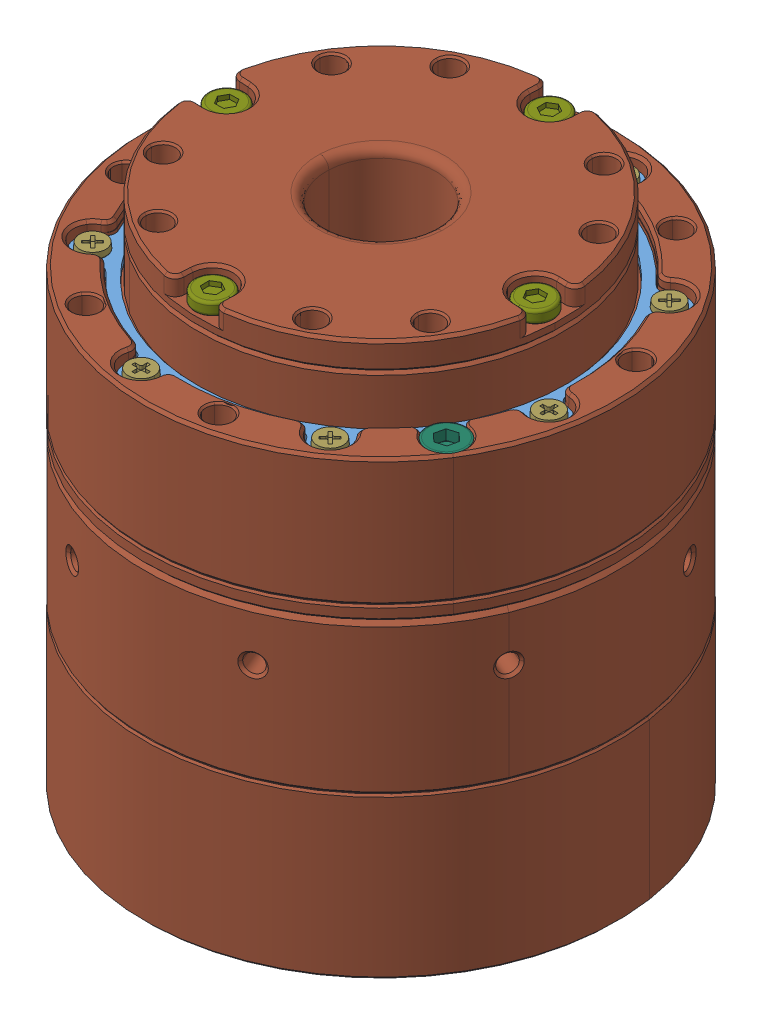
SolidWorks assembly CRA-RI40-52-PRO-XX 2023.5.4 - Drum, configuration 默认. Lengths in mm.
Overall size (67.95 60.31 67.96).
56 component instances, 34 part files, 0 mates.
Components (placement in the parent):
- CRA-RI40-52-PRO-XX 2023.5.4 - Drum.stp-1: CRA-RI40-52-PRO-XX 2023.5.4 - Drum.stp [默认] at origin size (67.95 60.31 67.96)
  - CRA-RI40-52-PRO-XX_1_ASM.stp-1: CRA-RI40-52-PRO-XX_1_ASM.stp [默认] at origin size (67.95 60.31 67.96)
    - XB11-52__10001_ASM.stp-1: XB11-52__10001_ASM.stp [默认] at (0 16.8 0) x (0.703875 0 -0.710324) z (-0.710324 0 -0.703875) size (66.32 0.8 66.32)
      - XB11-52-06__10001.stp-1: XB11-52-06__10001.stp [默认] at (0 15.8 0) x (0.791272 0 -0.611464) z (-0.611464 0 -0.791272) size (47.28 0.81 47.28)
    - TINYMBS20WITHCONNECTOR2_ASM.stp-1: TINYMBS20WITHCONNECTOR2_ASM.stp [默认] at (2.7275 -27.9719 -6.5848) x (0 -1 0) z (0.92388 0 0.382683) size (0.82 3.25 5.53)
      - FH34SRJ8S05SH_STEP_STEP_ASM.stp-1: FH34SRJ8S05SH_STEP_STEP_ASM.stp [默认] at (-6.4719 -22.2833 0) x (0 0 -1) z (1 0 0) size (5.53 3.25 0.82)
        - NONE-51348.stp-1: NONE-51348.stp [默认] at origin size (0.15 0.3 0.08)
        - NONE-53783.stp-1: NONE-53783.stp [默认] at origin size (0.15 0.3 0.08)
        - NONE-55744.stp-1: NONE-55744.stp [默认] at origin size (0.15 0.08 0.08)
        - NONE-57763.stp-1: NONE-57763.stp [默认] at origin size (0.15 0.08 0.08)
        - NONE-60582.stp-1: NONE-60582.stp [默认] at origin size (0.15 0.3 0.08)
        - NONE-60979.stp-1: NONE-60979.stp [默认] at origin size (0.15 0.3 0.08)
        - NONE-62950.stp-1: NONE-62950.stp [默认] at origin size (0.15 0.3 0.08)
        - NONE-64179.stp-1: NONE-64179.stp [默认] at origin size (0.15 0.3 0.08)
        - NONE-65774.stp-1: NONE-65774.stp [默认] at origin size (0.15 0.08 0.08)
        - NONE-66548.stp-1: NONE-66548.stp [默认] at origin size (0.15 0.35 0.23)
        - NONE-67775.stp-1: NONE-67775.stp [默认] at origin size (0.15 0.35 0.23)
        - NONE-133224.stp-1: NONE-133224.stp [默认] at origin size (0.15 0.08 0.08)
        - NONE-134873.stp-1: NONE-134873.stp [默认] at origin size (0.15 0.3 0.08)
        - NONE-136443.stp-1: NONE-136443.stp [默认] at origin size (0.15 0.08 0.08)
        - NONE-141250.stp-1: NONE-141250.stp [默认] at origin size (0.15 0.35 0.23)
        - NONE-145287.stp-1: NONE-145287.stp [默认] at origin size (0.15 0.08 0.08)
        - NONE-147294.stp-1: NONE-147294.stp [默认] at origin size (0.15 0.08 0.08)
        - NONE-214429.stp-1: NONE-214429.stp [默认] at origin size (0.15 0.9 0.82)
        - NONE-214822.stp-1: NONE-214822.stp [默认] at origin size (0.15 0.3 0.08)
        - NONE-215190.stp-1: NONE-215190.stp [默认] at origin size (0.15 0.08 0.08)
        - NONE-216041.stp-1: NONE-216041.stp [默认] at origin size (0.15 0.35 0.23)
        - NONE-217624.stp-1: NONE-217624.stp [默认] at origin size (0.15 0.35 0.23)
        - NONE-222885.stp-1: NONE-222885.stp [默认] at origin size (0.15 0.35 0.23)
        - NONE-224875.stp-1: NONE-224875.stp [默认] at origin size (0.15 0.35 0.23)
        - NONE-228113.stp-1: NONE-228113.stp [默认] at origin size (0.15 0.9 0.82)
        - NONE-228916.stp-1: NONE-228916.stp [默认] at origin size (0.15 0.35 0.23)
    - CROSS_RECESSED_COUNTERSUNK_HE_1.stp-1: CROSS_RECESSED_COUNTERSUNK_HE_1.stp [默认] at (-21.8123 -33.1 2.8703) x (0 1 0) z (0.6 0 0.8) size (4 3.5 3.5)
    - RI40-52-D12-02__1000.stp-1: RI40-52-D12-02__1000.stp [默认] at (0 -15 0) x (0.382683 0 -0.92388) z (0.92388 0 0.382683) size (52.01 56.6 52)
    - CROSS_RECESSED_CHEESE_HEAD_SC_1.stp-1: CROSS_RECESSED_CHEESE_HEAD_SC_1.stp [默认] at (3.9505 15.5 -22.4044) x (0 -1 0) z (1 0 0) size (5.7 2.98 2.98)
    - MC50-D25X12_5_000.stp-1: MC50-D25X12_5_000.stp [默认] at (0.0001 -26.6014 0.0001) x (0.382686 0 -0.923879) z (0 -1 0) size (48.11 50.01 13.43)
    - CROSS_RECESSED_CHEESE_HEAD_SC_1.stp-2: CROSS_RECESSED_CHEESE_HEAD_SC_1.stp [默认] at (-3.9505 15.5 22.4044) x (0 -1 0) z (-1 0 0) size (5.7 2.98 2.98)
    - CROSS_RECESSED_COUNTERSUNK_HE_1.stp-2: CROSS_RECESSED_COUNTERSUNK_HE_1.stp [默认] at (-3.0048 -33.1 22.5417) x (0 1 0) z (0.395734 0 0.918365) size (4 3.5 3.5)
    - CROSS_RECESSED_CHEESE_HEAD_SC_1.stp-3: CROSS_RECESSED_CHEESE_HEAD_SC_1.stp [默认] at (-18.6357 15.5 13.0489) x (0 -1 0) z (-0.707107 0 -0.707107) size (5.7 2.98 2.98)
    - CROSS_RECESSED_COUNTERSUNK_HE_1.stp-3: CROSS_RECESSED_COUNTERSUNK_HE_1.stp [默认] at (18.8645 -33.1 -12.4259) x (0 1 0) z (0.188455 0 0.982082) size (4 3.5 3.5)
    - _M2X3_M2X3_100.stp-1: _M2X3_M2X3_100.stp [默认] at (-21.8118 -29.6014 2.8705) x (0.8 0 -0.6) z (0.6 0 0.8) size (3.23 5.8 2.8)
    - _M2X3_M2X3_100.stp-2: _M2X3_M2X3_100.stp [默认] at (-13.393 -29.6014 -17.4539) x (0.918365 0 -0.395734) z (0.395734 0 0.918365) size (3.23 5.8 2.8)
    - CROSS_RECESSED_CHEESE_HEAD_SC_1.stp-4: CROSS_RECESSED_CHEESE_HEAD_SC_1.stp [默认] at (-22.4044 15.5 -3.9505) x (0 -1 0) z (0 0 -1) size (5.7 2.98 2.98)
    - CROSS_RECESSED_CHEESE_HEAD_SC_1.stp-5: CROSS_RECESSED_CHEESE_HEAD_SC_1.stp [默认] at (13.0489 15.5 18.6357) x (0 -1 0) z (-0.707107 0 0.707107) size (5.7 2.98 2.98)
    - HEXAGON_SOCKET_HEAD_CAP_SCREW_1.stp-1: HEXAGON_SOCKET_HEAD_CAP_SCREW_1.stp [默认] at (19.8197 15.9 12.6265) x (0 -1 0) z (-0.954517 0 0.298155) size (22.5 4.5 4.5)
    - M2-3_10001.stp-1: M2-3_10001.stp [默认] at (0.7742 21 -17.7331) x (0.020141 0 0.999797) z (-0.999797 0 0.020141) size (4 5.4 4)
    - HEXAGON_SOCKET_HEAD_CAP_SCREW_1.stp-2: HEXAGON_SOCKET_HEAD_CAP_SCREW_1.stp [默认] at (-19.8197 15.9 -12.6265) x (0 -1 0) z (0.954517 0 -0.298155) size (22.5 4.5 4.5)
    - CROSS_RECESSED_CHEESE_HEAD_SC_1.stp-6: CROSS_RECESSED_CHEESE_HEAD_SC_1.stp [默认] at (18.6357 15.5 -13.0489) x (0 -1 0) z (0.707107 0 0.707107) size (5.7 2.98 2.98)
    - M2-3_10001.stp-2: M2-3_10001.stp [默认] at (-17.7331 21 -0.7742) x (0.999797 0 -0.020141) z (0.020141 0 0.999797) size (4 5.4 4)
    - _M2X3_M2X3_100.stp-3: _M2X3_M2X3_100.stp [默认] at (-3.0038 -29.6014 22.5414) x (0.982082 0 -0.188455) z (0.188455 0 0.982082) size (3.23 5.8 2.8)
    - M2-3_10001.stp-3: M2-3_10001.stp [默认] at (-0.7742 21 17.7331) x (-0.020141 0 -0.999797) z (0.999797 0 -0.020141) size (4 5.4 4)
    - _M2X3_M2X3_100.stp-4: _M2X3_M2X3_100.stp [默认] at (18.8646 -29.6014 -12.4267) size (3.23 5.8 2.8)
    - CROSS_RECESSED_COUNTERSUNK_HE_1.stp-4: CROSS_RECESSED_COUNTERSUNK_HE_1.stp [默认] at (-13.393 -33.1 -17.4539) x (0 1 0) z (0 0 1) size (4 3.5 3.5)
    - M2-3_10001.stp-4: M2-3_10001.stp [默认] at (17.7331 21 0.7742) x (-0.999797 0 0.020141) z (-0.020141 0 -0.999797) size (4 5.4 4)
    - CROSS_RECESSED_CHEESE_HEAD_SC_1.stp-7: CROSS_RECESSED_CHEESE_HEAD_SC_1.stp [默认] at (22.4044 15.5 3.9505) x (0 -1 0) z (0 0 1) size (5.7 2.98 2.98)
    - CROSS_RECESSED_CHEESE_HEAD_SC_1.stp-8: CROSS_RECESSED_CHEESE_HEAD_SC_1.stp [默认] at (-13.0489 15.5 -18.6357) x (0 -1 0) z (0.707107 0 -0.707107) size (5.7 2.98 2.98)
